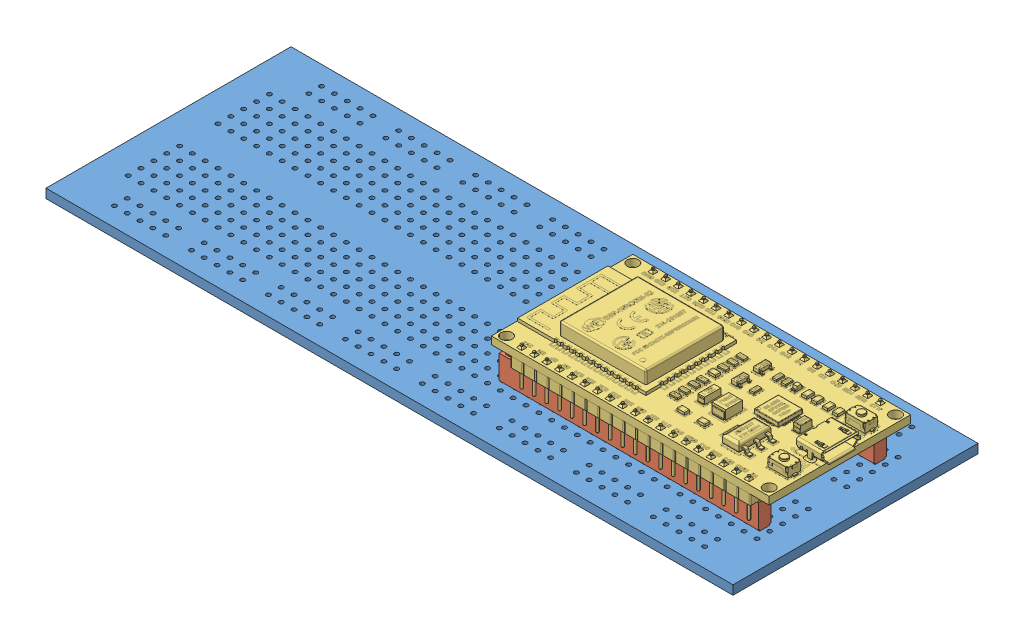
SolidWorks assembly ESP32_breadboard, configuration Predeterminado. Lengths in mm.
Overall size (136 14.62 48.5).
4 component instances, 3 part files, 9 mates.
Components (placement in the parent):
- placa breadboard-1: placa breadboard [Predeterminado] at (-172.7373 28.1214 24.25) size (136 1.8 48.5)
- 20-Pin Header - Female - 2.54mm-1: 20-Pin Header - Female - 2.54mm [Predeterminado] at (-93.0773 29.9214 11.43) size (51.3 8 2.5)
- 20-Pin Header - Female - 2.54mm-2: 20-Pin Header - Female - 2.54mm [Predeterminado] at (-93.0773 29.9214 -11.43) size (51.3 8 2.5)
- PCB_ESP32-38Pines-1: PCB_ESP32-38Pines [Predeterminado] at (-67.3173 36.9214 0) x (0 0 -1) z (1 0 0) size (28 10.12 55.48)
Mates (geometry in assembly coordinates):
- Ancho1: width: plane of 20-Pin Header - Female - 2.54mm-1 through (-44.4173 29.9214 11.43) normal (1 0 0); plane of 20-Pin Header - Female - 2.54mm-1 through (-45.2173 29.9214 11.43) normal (-1 0 0); cylinder of placa breadboard-1 through (-44.8173 29.9214 11.43) axis (0 -1 0) radius 0.425
- Ancho2: width: plane of 20-Pin Header - Female - 2.54mm-1 through (-45.2173 30.2214 11.755) normal (0 0 1); plane of 20-Pin Header - Female - 2.54mm-1 through (-45.2173 26.9214 11.105) normal (0 0 -1); cylinder of placa breadboard-1 through (-54.9773 29.9214 11.43) axis (0 -1 0) radius 0.425
- Ancho3: width: plane of 20-Pin Header - Female - 2.54mm-2 through (-45.2173 30.2214 -11.105) normal (0 0 1); plane of 20-Pin Header - Female - 2.54mm-2 through (-45.2173 26.9214 -11.755) normal (0 0 -1); cylinder of placa breadboard-1 through (-54.9773 29.9214 -11.43) axis (0 -1 0) radius 0.425
- Ancho4: width: plane of 20-Pin Header - Female - 2.54mm-2 through (-44.4173 29.9214 -11.43) normal (1 0 0); plane of 20-Pin Header - Female - 2.54mm-2 through (-45.2173 29.9214 -11.43) normal (-1 0 0); cylinder of placa breadboard-1 through (-44.8173 29.9214 -11.43) axis (0 -1 0) radius 0.425
- Coincidente1: coincident aligned: plane of 20-Pin Header - Female - 2.54mm-1 through (-94.5973 34.9214 10.18) normal (0 1 0); plane of 20-Pin Header - Female - 2.54mm-2 through (-94.5973 34.9214 -12.68) normal (0 1 0)
- Coincidente2: coincident anti-aligned: plane of placa breadboard-1 through (-172.7373 29.9214 24.25) normal (0 1 0); plane of 20-Pin Header - Female - 2.54mm-1 through (-94.5973 29.9214 12.68) normal (0 -1 0)
- Ancho5: width: plane of 20-Pin Header - Female - 2.54mm-2 through (-45.3173 29.9214 -11.43) normal (1 0 0); plane of 20-Pin Header - Female - 2.54mm-2 through (-44.3173 29.9214 -11.43) normal (-1 0 0); cylinder of PCB_ESP32-38Pines-1 through (-44.8173 38.4214 -13) axis (0 -1 0) radius 0.25
- Ancho6: width anti-aligned: plane of 20-Pin Header - Female - 2.54mm-2 through (-94.5973 29.9214 -12.68) normal (0 0 -1); plane of 20-Pin Header - Female - 2.54mm-1 through (-94.5973 34.9214 12.68) normal (0 0 1); plane of PCB_ESP32-38Pines-1 through (-94.8173 36.9214 14) normal (0 0 1); plane of PCB_ESP32-38Pines-1 through (-39.8173 36.9214 -14) normal (0 0 -1)
- Coincidente3: coincident anti-aligned: plane of 20-Pin Header - Female - 2.54mm-2 through (-94.5973 34.9214 -12.68) normal (0 1 0); plane of PCB_ESP32-38Pines-1 through (-44.8173 34.9214 -13) normal (0 -1 0)
